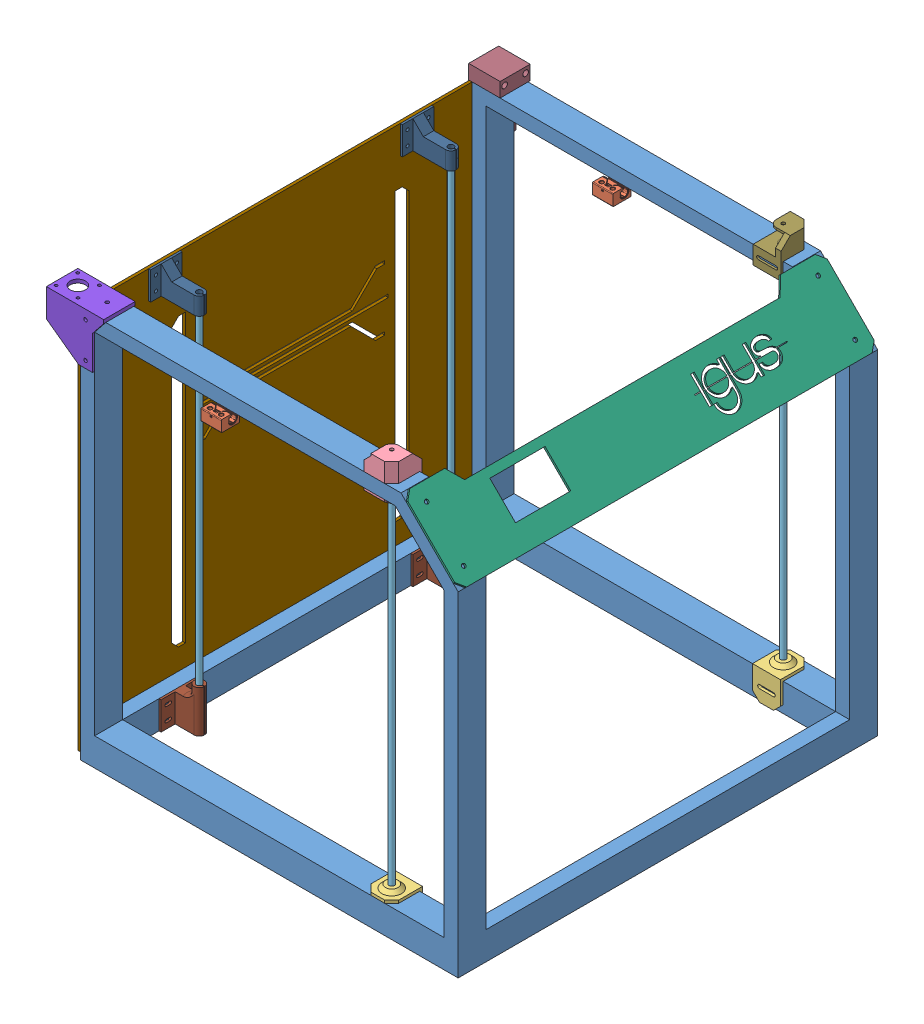
SolidWorks assembly Assem1, configuration Default. Lengths in mm.
Overall size (588.12 587.2 633).
26 component instances, 15 part files, 46 mates.
Components (placement in the parent):
- frame-1: frame [Default] at (-260.7928 -301.6494 -302.2349) size (540 560 600)
- Bearing-1: Bearing [Default] at (-43.1013 229.3506 257.7651) x (0 0 1) z (0 -1 0) size (26 29.76 16.5)
- Bearing-2: Bearing [Default] at (-72.1013 229.3506 297.7651) x (0 0 -1) z (0 -1 0) size (26 29.76 16.5)
- Bearing-3: Bearing [Default] at (-72.1013 229.3506 -262.2349) x (0 0 -1) z (0 -1 0) size (26 29.76 16.5)
- Bearing-4: Bearing [Default] at (-43.1013 229.3506 -302.2349) x (0 0 1) z (0 -1 0) size (26 29.76 16.5)
- plastic_holder_linear-2: plastic_holder_linear [Default] at (164.2072 -261.6494 277.7651) x (0 0 -1) z (1 0 0) size (44 48 40)
- plastic_holder_linear-4: plastic_holder_linear [Default] at (164.2072 -261.6494 -282.2349) x (0 0 1) z (-1 0 0) size (44 48 40)
- plastic_holder_linear_top_left-2: plastic_holder_linear_top_left [Default] at (164.2072 238.3506 277.7651) x (0 0 -1) z (-1 0 0) size (43 60.2 40)
- Linear_8mm-1: Linear_8mm [Default] at (-210.7928 -261.6494 178.0502) x (0.043288 0 -0.999063) z (0.999063 0 0.043288) size (8 500 8)
- Linear_8mm-2: Linear_8mm [Default] at (164.2072 -261.6494 -282.2349) size (8 500 8)
- Linear_8mm-3: Linear_8mm [Default] at (-210.7928 -261.6494 -181.9498) x (0.896674 0 -0.44269) z (0.44269 0 0.896674) size (8 500 8)
- Linear_8mm-4: Linear_8mm [Default] at (164.2072 -261.6494 277.7651) size (8 500 8)
- SheetMetal_front_cover-1: SheetMetal_front_cover [Default] at (197.8899 257.9521 302.3844) x (0 0 -1) z (0.707107 -0.707107 0) size (600 3 115)
- Rolamento Gt20-1: Rolamento Gt20 [Valor predeterminado] at (164.2072 262.3506 277.7651) x (0.263318 0 -0.964709) z (0.964709 0 0.263318) size (18 8.6 18)
- Rolamento Gt20-2: Rolamento Gt20 [Valor predeterminado] at (164.2072 273.9506 277.7651) x (0.996583 0 -0.082592) z (0.082592 0 0.996583) size (18 8.6 18)
- CoreXY_nema_fix-2: CoreXY_nema_fix [Default] at (-243.7928 258.3506 276.7651) x (0 0 -1) z (1 0 0) size (45 73.48 82)
- cover_back-1: cover_back [Default] at (-271.092 -9.9427 -33.0345) x (0 0 1) z (-1 0 0) size (600 560 57.34)
  - SheetMetal_back_cover-1: SheetMetal_back_cover [Default] at (-229.5201 169.8121 -10.2992) size (600 560 4)
  - PSupply-1: PSupply [Default] at (28.2576 -112.1123 -63.6392) x (0 1 0) z (0 0 -1) size (234.85 114.3 53.34) (hidden)
  - mks-1: mks [Default] at (28.5711 178.4658 -15.2992) x (1 0 0) z (0 1 0) size (144 22.79 85) (hidden)
- plastic_holder_rear_top-3: plastic_holder_rear_top [Default] at (-260.7928 258.3506 -189.4498) x (-1 0 0) z (0 0 1) size (57.5 40 45)
- plastic_holder_rear_top-4: plastic_holder_rear_top [Default] at (-260.7928 258.3506 170.5502) x (-1 0 0) z (0 0 1) size (57.5 40 45)
- plastic_holder_rear_bottom-1: plastic_holder_rear_bottom [Default] at (-240.7928 -301.6494 185.5502) x (-1 0 0) z (0 0 -1) size (37.5 60 55)
- plastic_holder_rear_bottom-2: plastic_holder_rear_bottom [Default] at (-240.7928 -301.6494 -174.4498) x (-1 0 0) z (0 0 -1) size (37.5 60 55)
- CoreXY_nema_fix_right-1: CoreXY_nema_fix_right [Default] at (164.2072 238.3506 -236.2349) x (0 0 -1) z (-1 0 0) size (43 60.2 40)
- nema-1: nema [Default] at (-262.7928 187.3506 -302.2349) x (-1 0 0) z (0 0 -1) size (45 91.5 43)
Mates (geometry in assembly coordinates):
- Parallel1: parallel aligned: plane of frame-1 through (-260.7928 258.3506 -262.2349) normal (0 1 0); plane of Bearing-4 through (-43.1013 236.8506 -311.2849) normal (0 1 0)
- Coincident9: coincident aligned: plane of Bearing-3 through (-43.1013 227.6999 -258.3992) normal (1 0 0); plane of Bearing-4 through (-43.1013 227.6999 -306.0707) normal (1 0 0)
- Parallel2: parallel aligned: plane of Bearing-3 through (-57.6013 220.3506 -262.1834) normal (0 -1 0); plane of Bearing-4 through (-57.6013 220.3506 -302.2865) normal (0 -1 0)
- Coincident11: coincident aligned: plane of Bearing-1 through (-43.1013 227.6999 253.9293) normal (1 0 0); plane of Bearing-4 through (-43.1013 227.6999 -306.0707) normal (1 0 0)
- Parallel3: parallel aligned: plane of frame-1 through (-260.7928 258.3506 257.7651) normal (0 1 0); plane of Bearing-1 through (-43.1013 236.8506 248.7151) normal (0 1 0)
- Coincident13: coincident aligned: plane of Bearing-1 through (-43.1013 227.6999 253.9293) normal (1 0 0); plane of Bearing-2 through (-43.1013 227.6999 301.6008) normal (1 0 0)
- Coincident14: coincident aligned: plane of Bearing-1 through (-43.1013 236.8506 248.7151) normal (0 1 0); plane of Bearing-2 through (-72.1013 236.8506 306.8151) normal (0 1 0)
- Coincident45: coincident anti-aligned: plane of frame-1 through (-260.7928 -301.6494 -262.2349) normal (0 0 1); plane of plastic_holder_linear-4 through (164.2072 -261.6494 -262.2349) normal (0 0 -1)
- Coincident50: coincident anti-aligned: plane of frame-1 through (-240.7928 238.3506 257.7651) normal (0 -1 0); plane of plastic_holder_linear_top_left-2 through (164.2072 238.3506 277.7651) normal (0 1 0)
- Coincident51: coincident anti-aligned: plane of frame-1 through (-260.7928 -301.6494 257.7651) normal (0 0 -1); plane of plastic_holder_linear_top_left-2 through (164.2072 238.3506 257.7651) normal (0 0 1)
- Concentric12: concentric anti-aligned: cylinder of plastic_holder_linear-2 through (164.2072 -257.6494 277.7651) axis (0 -1 0) radius 4; cylinder of plastic_holder_linear_top_left-2 through (164.2072 235.3506 277.7651) axis (0 1 0) radius 4.25
- Concentric13: concentric anti-aligned: circle of plastic_holder_linear-4; cylinder of Linear_8mm-2 through (164.2072 238.3506 -282.2349) axis (0 -1 0) radius 4
- Coincident54: coincident anti-aligned: plane of frame-1 through (-240.7928 238.3506 -262.2349) normal (0 -1 0); plane of Linear_8mm-2 through (164.2072 238.3506 -282.2349) normal (0 1 0)
- Coincident55: coincident anti-aligned: plane of frame-1 through (259.2072 -261.6494 -262.2349) normal (0 1 0); plane of Linear_8mm-3 through (-210.7928 -261.6494 -181.9498) normal (0 -1 0)
- Concentric15: concentric aligned: cylinder of plastic_holder_linear-2 through (164.2072 -257.6494 277.7651) axis (0 -1 0) radius 4; cylinder of Linear_8mm-4 through (164.2072 238.3506 277.7651) axis (0 -1 0) radius 4
- Coincident57: coincident anti-aligned: plane of frame-1 through (259.2072 -261.6494 257.7651) normal (0 1 0); plane of Linear_8mm-4 through (164.2072 -261.6494 277.7651) normal (0 -1 0)
- Coincident58: coincident anti-aligned: plane of frame-1 through (259.2072 -261.6494 257.7651) normal (0 1 0); plane of Linear_8mm-1 through (-210.7928 -261.6494 178.0502) normal (0 -1 0)
- Concentric23: concentric aligned: cylinder of plastic_holder_linear_top_left-2 through (164.2072 285.5506 277.7651) axis (0 -1 0) radius 2.5; cylinder of Rolamento Gt20-2 through (164.2072 273.9506 277.7651) axis (0 -1 0) radius 2.5
- Coincident78: coincident aligned: cylinder of plastic_holder_linear_top_left-2 through (164.2072 285.5506 277.7651) axis (0 -1 0) radius 2.5; circle of Rolamento Gt20-1
- Coincident80: coincident anti-aligned: plane of plastic_holder_linear_top_left-2 through (164.2072 262.3506 277.7651) normal (0 1 0); plane of Rolamento Gt20-1 through (163.0223 262.3506 282.1063) normal (0 -1 0)
- Coincident81: coincident anti-aligned: plane of plastic_holder_linear_top_left-2 through (164.2072 282.5506 277.7651) normal (0 -1 0); plane of Rolamento Gt20-2 through (155.2379 282.5506 278.5084) normal (0 1 0)
- Coincident83: coincident anti-aligned: plane of frame-1 through (-260.7928 258.3506 257.7651) normal (0 1 0); plane of CoreXY_nema_fix-2 through (-285.7928 258.3506 276.7651) normal (0 -1 0)
- Coincident88: coincident anti-aligned: plane of frame-1 through (197.4915 258.3506 257.7651) normal (0.707107 0.707107 0); plane of SheetMetal_front_cover-1 through (197.8899 257.9521 302.3844) normal (-0.707107 -0.707107 0)
- Coincident89: coincident aligned: plane of frame-1 through (-260.7928 -301.6494 297.7651) normal (0 0 1); plane of SheetMetal_front_cover-1 through (207.0823 253.0024 297.7651) normal (0 0 1)
- Coincident93: coincident anti-aligned: line of frame-1 through (279.2072 176.6349 257.7651) axis (0 0 1); line of SheetMetal_front_cover-1 through (279.2072 176.6349 287.7651) axis (0 0 -1)
- Coincident94: coincident anti-aligned: plane of frame-1 through (-260.7928 -301.6494 -262.2349) normal (-1 0 0); plane of cover_back-1/SheetMetal_back_cover-1 through (-260.7928 159.8694 -262.5547) normal (1 0 0)
- Coincident95: coincident aligned: plane of frame-1 through (-260.7928 -301.6494 -302.2349) normal (0 0 -1); plane of cover_back-1/SheetMetal_back_cover-1 through (-264.7928 -261.6494 -302.2349) normal (0 0 -1)
- Coincident96: coincident aligned: plane of frame-1 through (-260.7928 258.3506 -262.2349) normal (0 1 0); plane of cover_back-1/SheetMetal_back_cover-1 through (-264.7928 258.3506 -262.2349) normal (0 1 0)
- Concentric39: concentric aligned: cylinder of Linear_8mm-3 through (-210.7928 238.3506 -181.9498) axis (0 -1 0) radius 4; cylinder of plastic_holder_rear_top-3 through (-210.7928 258.3506 -181.9498) axis (0 -1 0) radius 4
- Parallel11: parallel anti-aligned: plane of cover_back-1/SheetMetal_back_cover-1 through (-260.7928 159.8694 -262.5547) normal (1 0 0); plane of plastic_holder_rear_top-3 through (-260.7928 258.3506 -174.4498) normal (-1 0 0)
- Coincident108: coincident: plane of Linear_8mm-3 through (-210.7928 238.3506 -181.9498) normal (0 1 0); plane of plastic_holder_rear_top-3 through (-210.7928 238.3506 -181.9498) normal (0 -1 0)
- Coincident109: coincident: plane of Linear_8mm-1 through (-210.7928 238.3506 178.0502) normal (0 1 0); plane of plastic_holder_rear_top-4 through (-210.7928 238.3506 178.0502) normal (0 -1 0)
- Concentric40: concentric aligned: cylinder of Linear_8mm-1 through (-210.7928 238.3506 178.0502) axis (0 -1 0) radius 4; cylinder of plastic_holder_rear_top-4 through (-210.7928 258.3506 178.0502) axis (0 -1 0) radius 4
- Parallel12: parallel anti-aligned: plane of cover_back-1/SheetMetal_back_cover-1 through (-260.7928 159.8694 -262.5547) normal (1 0 0); plane of plastic_holder_rear_top-4 through (-260.7928 258.3506 185.5502) normal (-1 0 0)
- Concentric43: concentric anti-aligned: cylinder of Linear_8mm-1 through (-210.7928 238.3506 178.0502) axis (0 -1 0) radius 4; cylinder of plastic_holder_rear_bottom-1 through (-210.7928 -306.6494 178.0502) axis (0 1 0) radius 4
- Parallel14: parallel anti-aligned: plane of frame-1 through (-240.7928 -301.6494 257.7651) normal (1 0 0); plane of plastic_holder_rear_bottom-1 through (-240.7928 -301.6494 170.5502) normal (-1 0 0)
- Coincident114: coincident aligned: plane of frame-1 through (279.2072 -301.6494 -262.2349) normal (0 -1 0); plane of plastic_holder_rear_bottom-1 through (-203.2928 -301.6494 170.5502) normal (0 -1 0)
- Coincident115: coincident aligned: plane of frame-1 through (279.2072 -301.6494 -262.2349) normal (0 -1 0); plane of plastic_holder_rear_bottom-2 through (-203.2928 -301.6494 -189.4498) normal (0 -1 0)
- Concentric44: concentric anti-aligned: cylinder of Linear_8mm-3 through (-210.7928 238.3506 -181.9498) axis (0 -1 0) radius 4; cylinder of plastic_holder_rear_bottom-2 through (-210.7928 -306.6494 -181.9498) axis (0 1 0) radius 4
- Parallel15: parallel anti-aligned: plane of frame-1 through (-240.7928 -301.6494 257.7651) normal (1 0 0); plane of plastic_holder_rear_bottom-2 through (-240.7928 -301.6494 -189.4498) normal (-1 0 0)
- Coincident119: coincident anti-aligned: plane of frame-1 through (-260.7928 258.3506 -262.2349) normal (0 1 0); plane of CoreXY_nema_fix_right-1 through (164.2072 258.3506 -282.2349) normal (0 -1 0)
- Coincident120: coincident anti-aligned: plane of frame-1 through (-260.7928 -301.6494 -262.2349) normal (0 0 1); plane of CoreXY_nema_fix_right-1 through (164.2072 238.3506 -262.2349) normal (0 0 -1)
- Coincident121: coincident aligned: plane of plastic_holder_linear_top_left-2 through (184.2072 235.3506 297.7651) normal (1 0 0); plane of CoreXY_nema_fix_right-1 through (184.2072 235.3506 -302.2349) normal (1 0 0)
- Coincident122: coincident anti-aligned: plane of frame-1 through (-260.7928 -301.6494 -302.2349) normal (0 0 -1); plane of nema-1 through (-240.7928 262.3506 -302.2349) normal (0 0 1)
- Coincident123: coincident anti-aligned: plane of frame-1 through (-260.7928 258.3506 -262.2349) normal (0 1 0); plane of nema-1 through (-262.7928 258.3506 -302.2349) normal (0 -1 0)
- Distance1: distance = 2 mm anti-aligned: plane of nema-1 through (-262.7928 262.3506 -302.2349) normal (1 0 0); plane of frame-1 through (-260.7928 -301.6494 -262.2349) normal (-1 0 0)
